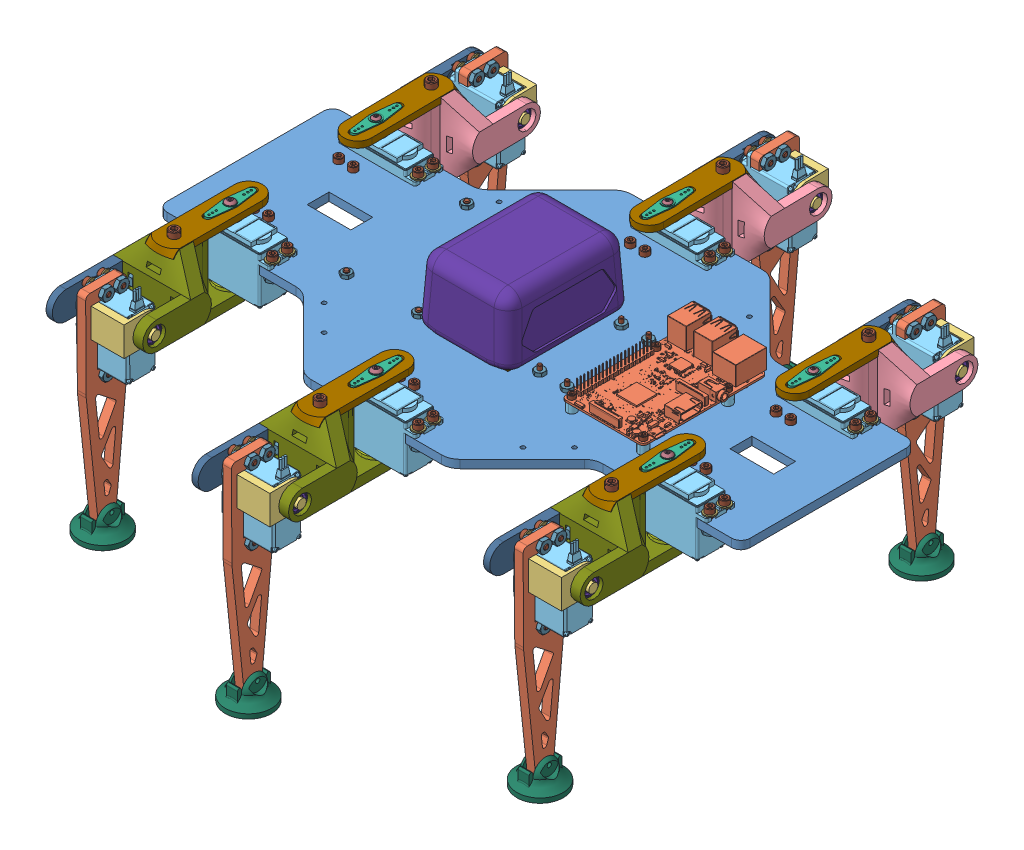
SolidWorks assembly Hexapod, configuration Défaut. Lengths in mm. (continued)
Components (placement in the parent): (continued)
- Battery-1: Battery [Défaut] at (-209.6397 14.6626 -46.247) x (-1 0 0) z (0 0 1) size (64.47 74.3 85.78)
  - MAKITA 4.0AH-1: MAKITA 4.0AH [Défaut] at (0.5853 -29.7874 85.4436) size (64.47 57.15 85.78)
  - MAKITA 4.0AH MOBILE-1: MAKITA 4.0AH MOBILE [Défaut] at (0.5853 -39.3124 91.7936) size (45.84 26.68 66.29)
- arduinoMega-1: arduinoMega [Detailed] at (-270.251 -7.6 40.62) x (0 0 -1) z (-1 0 0) size (108.32 14.5 53.3)
- raspberryPi3B-1: raspberryPi3B [Detailed] at (-112.5 6.35 40) x (0 0 -1) z (0 1 0) size (87.05 58.5 19.5)
- 12Channel PWM-1: 12Channel PWM [Default] at (-160.6 -5.6 40) x (-1 0 0) z (0 0 1) size (25.4 7.55 66.7)
- DROK_090483.stp-1: DROK_090483.stp [Default] at (-90.995 -5.6 69.895) x (-1 0 0) z (0 -1 0) size (50.02 60 18.9)
- socket head cap screw_ai-2: socket head cap screw_ai [HX-SHCS 0.138-32x0.625x0.625-N] at (-54.94 3.5052 69.09) x (0 -1 0) z (1 0 0) size (19.38 5.74 5.74)
- socket head cap screw_ai-3: socket head cap screw_ai [HX-SHCS 0.138-32x0.625x0.625-N] at (-64.94 3.5052 69.09) x (0 -1 0) z (0.5 0 0.866025) size (19.38 5.74 5.74)
- socket head cap screw_ai-4: socket head cap screw_ai [HX-SHCS 0.138-32x0.625x0.625-N] at (-64.94 3.5052 10.91) x (0 -1 0) z (1 0 0) size (19.38 5.74 5.74)
- socket head cap screw_ai-5: socket head cap screw_ai [HX-SHCS 0.138-32x0.625x0.625-N] at (-54.94 3.5052 10.91) x (0 -1 0) z (1 0 0) size (19.38 5.74 5.74)
- socket head cap screw_ai-6: socket head cap screw_ai [HX-SHCS 0.138-32x0.625x0.625-N] at (-214.94 3.5052 119.09) x (0 -1 0) z (1 0 0) size (19.38 5.74 5.74)
- socket head cap screw_ai-7: socket head cap screw_ai [HX-SHCS 0.138-32x0.625x0.625-N] at (-204.94 3.5052 119.09) x (0 -1 0) z (1 0 0) size (19.38 5.74 5.74)
- socket head cap screw_ai-14: socket head cap screw_ai [HX-SHCS 0.138-32x0.625x0.625-N] at (-204.94 3.5052 -39.09) x (0 -1 0) z (1 0 0) size (19.38 5.74 5.74)
- socket head cap screw_ai-15: socket head cap screw_ai [HX-SHCS 0.138-32x0.625x0.625-N] at (-214.94 3.5052 -39.09) x (0 -1 0) z (1 0 0) size (19.38 5.74 5.74)
- socket head cap screw_ai-16: socket head cap screw_ai [HX-SHCS 0.138-32x0.625x0.625-N] at (-354.94 3.5052 69.09) x (0 -1 0) z (1 0 0) size (19.38 5.74 5.74)
- socket head cap screw_ai-17: socket head cap screw_ai [HX-SHCS 0.138-32x0.625x0.625-N] at (-364.94 3.5052 69.09) x (0 -1 0) z (0.5 0 0.866025) size (19.38 5.74 5.74)
- socket head cap screw_ai-18: socket head cap screw_ai [HX-SHCS 0.138-32x0.625x0.625-N] at (-364.94 3.5052 10.91) x (0 -1 0) z (1 0 0) size (19.38 5.74 5.74)
- socket head cap screw_ai-19: socket head cap screw_ai [HX-SHCS 0.138-32x0.625x0.625-N] at (-354.94 3.5052 10.91) x (0 -1 0) z (1 0 0) size (19.38 5.74 5.74)
- machine screw nut hex_ai-60: machine screw nut hex_ai [MSHXNUT 0.138-32-D-N] at (-373.75 -8.4956 -15.08) x (1 0 0) z (0 -1 0) size (7.92 9.15 2.9)
- machine screw nut hex_ai-65: machine screw nut hex_ai [MSHXNUT 0.138-32-D-N] at (-373.75 -8.4956 -4.92) x (1 0 0) z (0 -1 0) size (7.92 9.15 2.9)
- machine screw nut hex_ai-70: machine screw nut hex_ai [MSHXNUT 0.138-32-D-N] at (-326.252 -8.4956 -4.92) x (0.5 0 0.866025) z (0 -1 0) size (7.92 9.15 2.9)
- machine screw nut hex_ai-75: machine screw nut hex_ai [MSHXNUT 0.138-32-D-N] at (-326.252 -8.4956 -15.08) x (0.5 0 0.866025) z (0 -1 0) size (7.92 9.15 2.9)
- machine screw nut hex_ai-80: machine screw nut hex_ai [MSHXNUT 0.138-32-D-N] at (-354.94 -13.5656 10.91) x (0 0 1) z (0 -1 0) size (7.92 9.15 2.9)
- machine screw nut hex_ai-85: machine screw nut hex_ai [MSHXNUT 0.138-32-D-N] at (-364.94 -13.5656 10.91) x (0 0 1) z (0 -1 0) size (7.92 9.15 2.9)
- machine screw nut hex_ai-63: machine screw nut hex_ai [MSHXNUT 0.138-32-D-N] at (-223.75 -8.4956 -65.08) x (1 0 0) z (0 -1 0) size (7.92 9.15 2.9)
- machine screw nut hex_ai-68: machine screw nut hex_ai [MSHXNUT 0.138-32-D-N] at (-223.75 -8.4956 -54.92) x (1 0 0) z (0 -1 0) size (7.92 9.15 2.9)
- machine screw nut hex_ai-73: machine screw nut hex_ai [MSHXNUT 0.138-32-D-N] at (-176.252 -8.4956 -54.92) x (0.5 0 0.866025) z (0 -1 0) size (7.92 9.15 2.9)
- machine screw nut hex_ai-78: machine screw nut hex_ai [MSHXNUT 0.138-32-D-N] at (-176.252 -8.4956 -65.08) x (0.5 0 0.866025) z (0 -1 0) size (7.92 9.15 2.9)
- machine screw nut hex_ai-83: machine screw nut hex_ai [MSHXNUT 0.138-32-D-N] at (-204.94 -13.5656 -39.09) x (0 0 1) z (0 -1 0) size (7.92 9.15 2.9)
- machine screw nut hex_ai-86: machine screw nut hex_ai [MSHXNUT 0.138-32-D-N] at (-214.94 -13.5656 -39.09) x (0 0 1) z (0 -1 0) size (7.92 9.15 2.9)
- machine screw nut hex_ai-87: machine screw nut hex_ai [MSHXNUT 0.138-32-D-N] at (-64.94 -13.5656 10.91) x (0 0 1) z (0 -1 0) size (7.92 9.15 2.9)
- machine screw nut hex_ai-84: machine screw nut hex_ai [MSHXNUT 0.138-32-D-N] at (-54.94 -13.5656 10.91) x (0 0 1) z (0 -1 0) size (7.92 9.15 2.9)
- machine screw nut hex_ai-74: machine screw nut hex_ai [MSHXNUT 0.138-32-D-N] at (-26.252 -8.4956 -4.92) x (0.5 0 0.866025) z (0 -1 0) size (7.92 9.15 2.9)
- machine screw nut hex_ai-79: machine screw nut hex_ai [MSHXNUT 0.138-32-D-N] at (-26.252 -8.4956 -15.08) x (0.5 0 0.866025) z (0 -1 0) size (7.92 9.15 2.9)
- machine screw nut hex_ai-69: machine screw nut hex_ai [MSHXNUT 0.138-32-D-N] at (-73.75 -8.4956 -4.92) x (1 0 0) z (0 -1 0) size (7.92 9.15 2.9)
- machine screw nut hex_ai-64: machine screw nut hex_ai [MSHXNUT 0.138-32-D-N] at (-73.75 -8.4956 -15.08) x (1 0 0) z (0 -1 0) size (7.92 9.15 2.9)
- machine screw nut hex_ai-88: machine screw nut hex_ai [MSHXNUT 0.138-32-D-N] at (-364.94 -10.67 69.09) x (0 0 -1) z (0 1 0) size (7.92 9.15 2.9)
- machine screw nut hex_ai-89: machine screw nut hex_ai [MSHXNUT 0.138-32-D-N] at (-354.94 -10.67 69.09) x (0 0 -1) z (0 1 0) size (7.92 9.15 2.9)
- machine screw nut hex_ai-90: machine screw nut hex_ai [MSHXNUT 0.138-32-D-N] at (-326.252 -5.6 84.92) x (0.5 0 -0.866025) z (0 1 0) size (7.92 9.15 2.9)
- machine screw nut hex_ai-91: machine screw nut hex_ai [MSHXNUT 0.138-32-D-N] at (-326.252 -5.6 95.08) x (0.5 0 -0.866025) z (0 1 0) size (7.92 9.15 2.9)
- machine screw nut hex_ai-92: machine screw nut hex_ai [MSHXNUT 0.138-32-D-N] at (-373.75 -5.6 84.92) x (1 0 0) z (0 1 0) size (7.92 9.15 2.9)
- machine screw nut hex_ai-93: machine screw nut hex_ai [MSHXNUT 0.138-32-D-N] at (-373.75 -5.6 95.08) x (1 0 0) z (0 1 0) size (7.92 9.15 2.9)
- machine screw nut hex_ai-94: machine screw nut hex_ai [MSHXNUT 0.138-32-D-N] at (-223.75 -5.6 145.08) x (1 0 0) z (0 1 0) size (7.92 9.15 2.9)
- machine screw nut hex_ai-95: machine screw nut hex_ai [MSHXNUT 0.138-32-D-N] at (-223.75 -5.6 134.92) x (1 0 0) z (0 1 0) size (7.92 9.15 2.9)
- machine screw nut hex_ai-96: machine screw nut hex_ai [MSHXNUT 0.138-32-D-N] at (-176.252 -5.6 134.92) x (0.5 0 -0.866025) z (0 1 0) size (7.92 9.15 2.9)
- machine screw nut hex_ai-97: machine screw nut hex_ai [MSHXNUT 0.138-32-D-N] at (-176.252 -5.6 145.08) x (0.5 0 -0.866025) z (0 1 0) size (7.92 9.15 2.9)
- machine screw nut hex_ai-98: machine screw nut hex_ai [MSHXNUT 0.138-32-D-N] at (-204.94 -10.67 119.09) x (0 0 -1) z (0 1 0) size (7.92 9.15 2.9)
- machine screw nut hex_ai-99: machine screw nut hex_ai [MSHXNUT 0.138-32-D-N] at (-214.94 -10.67 119.09) x (0 0 -1) z (0 1 0) size (7.92 9.15 2.9)
- machine screw nut hex_ai-100: machine screw nut hex_ai [MSHXNUT 0.138-32-D-N] at (-64.94 -10.67 69.09) x (0 0 -1) z (0 1 0) size (7.92 9.15 2.9)
- machine screw nut hex_ai-101: machine screw nut hex_ai [MSHXNUT 0.138-32-D-N] at (-54.94 -10.67 69.09) x (0 0 -1) z (0 1 0) size (7.92 9.15 2.9)
- machine screw nut hex_ai-102: machine screw nut hex_ai [MSHXNUT 0.138-32-D-N] at (-26.252 -5.6 84.92) x (0.5 0 -0.866025) z (0 1 0) size (7.92 9.15 2.9)
- machine screw nut hex_ai-103: machine screw nut hex_ai [MSHXNUT 0.138-32-D-N] at (-26.252 -5.6 95.08) x (0.5 0 -0.866025) z (0 1 0) size (7.92 9.15 2.9)
- machine screw nut hex_ai-104: machine screw nut hex_ai [MSHXNUT 0.138-32-D-N] at (-73.75 -5.6 84.92) x (1 0 0) z (0 1 0) size (7.92 9.15 2.9)
- machine screw nut hex_ai-105: machine screw nut hex_ai [MSHXNUT 0.138-32-D-N] at (-73.75 -5.6 95.08) x (1 0 0) z (0 1 0) size (7.92 9.15 2.9)
- socket head cap screw_ai-20: socket head cap screw_ai [HX-SHCS 0.138-32x0.5x0.5-N] at (-246.141 -12.6052 74.88) x (0 1 0) z (-0.5 0 -0.866025) size (16.21 5.74 5.74)
- socket head cap screw_ai-21: socket head cap screw_ai [HX-SHCS 0.138-32x0.5x0.5-N] at (-294.361 -12.6052 -6.36) x (0 1 0) z (1 0 0) size (16.21 5.74 5.74)
- socket head cap screw_ai-22: socket head cap screw_ai [HX-SHCS 0.138-32x0.5x0.5-N] at (-246.141 -12.6052 0) x (0 1 0) z (-0.5 0 -0.866025) size (16.21 5.74 5.74)
- socket head cap screw_ai-23: socket head cap screw_ai [HX-SHCS 0.138-32x0.5x0.5-N] at (-294.361 -12.6052 76.11) x (0 1 0) z (-1 0 0) size (16.21 5.74 5.74)
- machine screw nut hex_ai-106: machine screw nut hex_ai [MSHXNUT 0.112-40-D-N] at (-294.361 2.4892 -6.36) x (1 0 0) z (0 1 0) size (6.35 7.33 2.49)
- machine screw nut hex_ai-107: machine screw nut hex_ai [MSHXNUT 0.112-40-D-N] at (-294.361 2.4892 76.11) x (1 0 0) z (0 1 0) size (6.35 7.33 2.49)
- machine screw nut hex_ai-108: machine screw nut hex_ai [MSHXNUT 0.112-40-D-N] at (-246.141 2.4892 0) x (1 0 0) z (0 1 0) size (6.35 7.33 2.49)
- machine screw nut hex_ai-109: machine screw nut hex_ai [MSHXNUT 0.112-40-D-N] at (-246.141 2.4892 74.88) x (1 0 0) z (0 1 0) size (6.35 7.33 2.49)
- socket head cap screw_ai-24: socket head cap screw_ai [HX-SHCS 0.138-32x0.5x0.5-N] at (-130.81 -10.3052 13.48) x (0 1 0) z (-0.5 0 -0.866025) size (16.21 5.74 5.74)
- machine screw nut hex_ai-110: machine screw nut hex_ai [MSHXNUT 0.112-40-D-N] at (-130.81 2.4892 13.48) x (1 0 0) z (0 1 0) size (6.35 7.33 2.49)
- socket head cap screw_ai-25: socket head cap screw_ai [HX-SHCS 0.138-32x0.5x0.5-N] at (-94.18 -10.3052 13.48) x (0 1 0) z (-0.5 0 -0.866025) size (16.21 5.74 5.74)
- socket head cap screw_ai-26: socket head cap screw_ai [HX-SHCS 0.138-32x0.5x0.5-N] at (-130.81 -10.3052 66.31) x (0 1 0) z (-0.5 0 -0.866025) size (16.21 5.74 5.74)
- socket head cap screw_ai-27: socket head cap screw_ai [HX-SHCS 0.138-32x0.5x0.5-N] at (-94.18 -10.3052 66.31) x (0 1 0) z (-0.5 0 -0.866025) size (16.21 5.74 5.74)
- machine screw nut hex_ai-111: machine screw nut hex_ai [MSHXNUT 0.112-40-D-N] at (-94.18 2.4892 13.48) x (1 0 0) z (0 1 0) size (6.35 7.33 2.49)
- machine screw nut hex_ai-112: machine screw nut hex_ai [MSHXNUT 0.112-40-D-N] at (-130.81 2.4892 66.31) x (1 0 0) z (0 1 0) size (6.35 7.33 2.49)
- machine screw nut hex_ai-113: machine screw nut hex_ai [MSHXNUT 0.112-40-D-N] at (-94.18 2.4892 66.31) x (1 0 0) z (0 1 0) size (6.35 7.33 2.49)
- 1_4_Round_Aluminum_Standoff.step-1: 1_4_Round_Aluminum_Standoff.step [Défaut] at (-88 0 21) x (0.963282 0 -0.268492) z (0.268492 0 0.963282) size (6.34 6.36 6.34)
- socket head cap screw_ai-28: socket head cap screw_ai [HX-SHCS 0.112-40x1x0.75-N] at (-88 10.4948 21) x (0 -1 0) z (0.5 0 0.866025) size (28.24 4.65 4.65)
- machine screw nut hex_ai-114: machine screw nut hex_ai [MSHXNUT 0.112-40-D-N] at (-88 -8.0892 21) x (1 0 0) z (0 -1 0) size (6.35 7.33 2.49)
- 1_4_Round_Aluminum_Standoff.step-2: 1_4_Round_Aluminum_Standoff.step [Défaut] at (-137 0 21) x (0.963282 0 -0.268492) z (0.268492 0 0.963282) size (6.34 6.36 6.34)
- 1_4_Round_Aluminum_Standoff.step-3: 1_4_Round_Aluminum_Standoff.step [Défaut] at (-88 0 79) x (0.963282 0 -0.268492) z (0.268492 0 0.963282) size (6.34 6.36 6.34)
- 1_4_Round_Aluminum_Standoff.step-4: 1_4_Round_Aluminum_Standoff.step [Défaut] at (-137 0 79) x (0.963282 0 -0.268492) z (0.268492 0 0.963282) size (6.34 6.36 6.34)
- machine screw nut hex_ai-115: machine screw nut hex_ai [MSHXNUT 0.112-40-D-N] at (-137 -8.0892 21) x (1 0 0) z (0 -1 0) size (6.35 7.33 2.49)
- machine screw nut hex_ai-116: machine screw nut hex_ai [MSHXNUT 0.112-40-D-N] at (-88 -8.0892 79) x (1 0 0) z (0 -1 0) size (6.35 7.33 2.49)
- machine screw nut hex_ai-117: machine screw nut hex_ai [MSHXNUT 0.112-40-D-N] at (-137 -8.0892 79) x (1 0 0) z (0 -1 0) size (6.35 7.33 2.49)
- socket head cap screw_ai-29: socket head cap screw_ai [HX-SHCS 0.112-40x1x0.75-N] at (-137 10.4948 21) x (0 -1 0) z (0.5 0 0.866025) size (28.24 4.65 4.65)
- socket head cap screw_ai-30: socket head cap screw_ai [HX-SHCS 0.112-40x1x0.75-N] at (-88 10.4948 79) x (0 -1 0) z (0.5 0 0.866025) size (28.24 4.65 4.65)
- socket head cap screw_ai-31: socket head cap screw_ai [HX-SHCS 0.112-40x1x0.75-N] at (-137 10.4948 79) x (0 -1 0) z (0.5 0 0.866025) size (28.24 4.65 4.65)
- socket head cap screw_ai-32: socket head cap screw_ai [HX-SHCS 0.112-40x0.5x0.5-N] at (-170 -9.9448 12.05) x (0 1 0) z (-1 0 0) size (15.54 4.65 4.65)
- machine screw nut hex_ai-118: machine screw nut hex_ai [MSHXNUT 0.112-40-D-N] at (-170 2.4892 12.05) x (1 0 0) z (0 1 0) size (6.35 7.33 2.49)
- socket head cap screw_ai-33: socket head cap screw_ai [HX-SHCS 0.112-40x0.5x0.5-N] at (-151.2 -9.9448 12.05) x (0 1 0) z (-1 0 0) size (15.54 4.65 4.65)
- socket head cap screw_ai-34: socket head cap screw_ai [HX-SHCS 0.112-40x0.5x0.5-N] at (-170 -9.9448 67.95) x (0 1 0) z (-1 0 0) size (15.54 4.65 4.65)
- socket head cap screw_ai-35: socket head cap screw_ai [HX-SHCS 0.112-40x0.5x0.5-N] at (-151.2 -9.9448 67.95) x (0 1 0) z (-1 0 0) size (15.54 4.65 4.65)
- machine screw nut hex_ai-119: machine screw nut hex_ai [MSHXNUT 0.112-40-D-N] at (-151.2 2.4892 12.05) x (1 0 0) z (0 1 0) size (6.35 7.33 2.49)
- machine screw nut hex_ai-120: machine screw nut hex_ai [MSHXNUT 0.112-40-D-N] at (-170 2.4892 67.95) x (1 0 0) z (0 1 0) size (6.35 7.33 2.49)
- machine screw nut hex_ai-121: machine screw nut hex_ai [MSHXNUT 0.112-40-D-N] at (-151.2 2.4892 67.95) x (1 0 0) z (0 1 0) size (6.35 7.33 2.49)
Mates (geometry in assembly coordinates):
- Coincident2: coincident anti-aligned: plane of Body-1 through (-370 -5.601 0) normal (0 0 -1)
- Coincident3: coincident aligned: plane of Body-1 through (-400 0 40) normal (0 1 0)
- Coincident4: coincident aligned: plane of Body-1 through (0 0 100) normal (1 0 0)
- Coincident5: coincident anti-aligned: plane of Body-1 through (-400 0 40) normal (0 1 0); plane of Assembly_Leg_V4-1/hs-422-3 through (-50.001 0 -0.094) normal (0 -1 0)
- Concentric3: concentric anti-aligned: cylinder of Body-1 through (-73.75 0 -15.08) axis (0 -1 0) radius 1.45; cylinder of Assembly_Leg_V4-1/hs-422-3 through (-73.75 -26.67 -15.08) axis (0 1 0) radius 2.1844
- Concentric6: concentric aligned: cylinder of Body-1 through (-373.75 -5.601 -4.92) axis (0 1 0) radius 1.45; cylinder of Assembly_Leg_V4-2/hs-422-3 through (-373.75 -26.67 -4.92) axis (0 1 0) radius 2.1844
- Parallel4: parallel anti-aligned: plane of Body-1 through (-370 -5.601 0) normal (0 0 -1); plane of Assembly_Leg_V4-2/hs-422-3 through (-350.001 -5.969 -0.094) normal (0 0 1)
- Coincident9: coincident anti-aligned: plane of Body-1 through (-400 0 40) normal (0 1 0); plane of Assembly_Leg_V4-2/hs-422-3 through (-350.001 0 -0.094) normal (0 -1 0)
- Coincident10: coincident anti-aligned: plane of Body-1 through (-400 0 40) normal (0 1 0); plane of Assembly_Leg_V4-3/hs-422-3 through (-200.001 0 -50.094) normal (0 -1 0)
- Concentric7: concentric anti-aligned: cylinder of Body-1 through (-223.75 0 -54.92) axis (0 -1 0) radius 1.45; cylinder of Assembly_Leg_V4-3/hs-422-3 through (-223.75 -26.67 -54.92) axis (0 1 0) radius 2.1844
- Parallel5: parallel anti-aligned: plane of Body-1 through (-220 -5.6 -50) normal (0 0 -1); plane of Assembly_Leg_V4-3/hs-422-3 through (-200.001 -5.969 -50.094) normal (0 0 1)
- Parallel6: parallel anti-aligned: plane of Body-1 through (-70 -5.6 0) normal (0 0 -1); plane of Assembly_Leg_V4-1/hs-422-3 through (-50.001 -5.969 -0.094) normal (0 0 1)
- Coincident11: coincident anti-aligned: plane of Body-1 through (-400 0 40) normal (0 1 0); plane of Assembly_Leg_V4_Mirror-1/hs-422-3 through (-350.001 0 99.906) normal (0 -1 0)
- Concentric8: concentric aligned: cylinder of Body-1 through (-373.75 -5.601 95.08) axis (0 1 0) radius 1.45; cylinder of Assembly_Leg_V4_Mirror-1/hs-422-3 through (-373.75 -26.67 95.08) axis (0 1 0) radius 2.1844
- Parallel7: parallel anti-aligned: plane of Body-1 through (-370 -5.601 80) normal (0 0 1); plane of Assembly_Leg_V4_Mirror-1/hs-422-3 through (-350.001 -5.969 80.094) normal (0 0 -1)
- Coincident13: coincident anti-aligned: plane of Body-1 through (-400 0 40) normal (0 1 0); plane of Assembly_Leg_V4_Mirror-2/hs-422-3 through (-50.001 0 99.906) normal (0 -1 0)
- Concentric9: concentric anti-aligned: cylinder of Body-1 through (-73.75 0 95.08) axis (0 -1 0) radius 1.45; cylinder of Assembly_Leg_V4_Mirror-2/hs-422-3 through (-73.75 -26.67 95.08) axis (0 1 0) radius 2.1844
- Parallel8: parallel anti-aligned: plane of Body-1 through (-70 -5.6 80) normal (0 0 1); plane of Assembly_Leg_V4_Mirror-2/hs-422-3 through (-50.001 -5.969 80.094) normal (0 0 -1)
- Coincident15: coincident anti-aligned: plane of Body-1 through (-400 0 40) normal (0 1 0); plane of Assembly_Leg_V4_Mirror-3/hs-422-3 through (-200.001 0 149.906) normal (0 -1 0)
- Concentric10: concentric anti-aligned: cylinder of Body-1 through (-223.75 0 145.08) axis (0 -1 0) radius 1.45; cylinder of Assembly_Leg_V4_Mirror-3/hs-422-3 through (-223.75 -26.67 145.08) axis (0 1 0) radius 2.1844
- Parallel9: parallel anti-aligned: plane of Body-1 through (-220 -5.6 130) normal (0 0 1); plane of Assembly_Leg_V4_Mirror-3/hs-422-3 through (-200.001 -5.969 130.094) normal (0 0 -1)
- Coïncidente1: coincident anti-aligned: plane of Body-1 through (-400 0 40) normal (0 1 0); plane of Batterie-1/MAKITA 4.0AH-1 through (-210.225 0 39.1966) normal (0 -1 0)
- Coïncidente2: coincident anti-aligned: plane of arduinoMega-1 through (-270.251 -5.6 40.62) normal (0 1 0); plane of Body-1 through (-400 -5.6 40) normal (0 -1 0)
- Coïncidente4: coincident anti-aligned: plane of Body-1 through (-400 -5.6 40) normal (0 -1 0); plane of 12Channel PWM-1 through (-170 -5.6 12.05) normal (0 1 0)
- Coïncidente5: coincident anti-aligned: plane of Body-1 through (-400 -5.6 40) normal (0 -1 0); plane of DROK_090483.stp-1 through (-112.495 -5.6 39.895) normal (0 1 0)
- Parallèle4: parallel aligned: plane of Body-1 through (0 0 100) normal (1 0 0); plane of 12Channel PWM-1 through (-147.9 -7.1 12.05) normal (1 0 0)
- Concentric13: concentric aligned: cylinder of Body-1 through (-170 0 67.95) axis (0 -1 0) radius 1.25; cylinder of 12Channel PWM-1 through (-170 -2.0645 67.95) axis (0 -1 0) radius 1.25
- Concentric15: concentric aligned: cylinder of Body-1 through (-137 -5.6 21) axis (0 1 0) radius 1.375; cylinder of raspberryPi3B-1 through (-137 6.35 21) axis (0 1 0) radius 1.375
- Concentric16: concentric aligned: cylinder of Body-1 through (-88 -5.6 79) axis (0 1 0) radius 1.375; cylinder of raspberryPi3B-1 through (-88 6.35 79) axis (0 1 0) radius 1.375
- Coincident17: coincident anti-aligned: plane of Body-1 through (-232.45 0 2.16) normal (1 0 0); plane of Batterie-1/MAKITA 4.0AH MOBILE-1 through (-232.45 53.975 45.5466) normal (-1 0 0)
- Coincident18: coincident anti-aligned: plane of Body-1 through (-232.45 0 77.85) normal (0 0 -1); plane of Batterie-1/MAKITA 4.0AH MOBILE-1 through (-192.7625 -22.225 77.85) normal (0 0 1)
- Concentric17: concentric anti-aligned: circle of Body-1; circle of DROK_090483.stp-1
- Concentric18: concentric aligned: cylinder of Body-1 through (-94.18 0 66.31) axis (0 -1 0) radius 1.45; cylinder of DROK_090483.stp-1 through (-94.18 -5.6 66.31) axis (0 -1 0) radius 1.585
- Concentric19: concentric aligned: cylinder of Body-1 through (-246.141 0 0) axis (0 -1 0) radius 1.6; circle of arduinoMega-1
- Concentric22: concentric aligned: cylinder of Body-1 through (-294.361 0 76.11) axis (0 -1 0) radius 1.6; cylinder of arduinoMega-1 through (-294.361 -7.6 76.11) axis (0 -1 0) radius 1.6
- Concentric23: concentric anti-aligned: cylinder of Body-1 through (-54.94 0 69.09) axis (0 -1 0) radius 1.45; cylinder of HX-SHCS 0.138-32x0.625x0.625-N-2 through (-54.94 35.2552 69.09) axis (0 1 0) radius 1.7526
- Concentric24: concentric anti-aligned: cylinder of Body-1 through (-64.94 0 69.09) axis (0 -1 0) radius 1.45; cylinder of HX-SHCS 0.138-32x0.625x0.625-N-3 through (-64.94 35.2552 69.09) axis (0 1 0) radius 1.7526
- Coincident19: coincident anti-aligned: plane of Body-1 through (-400 0 40) normal (0 1 0); plane of HX-SHCS 0.138-32x0.625x0.625-N-2 through (-54.94 0 66.2198) normal (0 -1 0)
- Coincident20: coincident anti-aligned: plane of Body-1 through (-400 0 40) normal (0 1 0); plane of HX-SHCS 0.138-32x0.625x0.625-N-3 through (-62.4543 0 67.6549) normal (0 -1 0)
- Parallel10: parallel aligned: plane of Body-1 through (0 0 100) normal (1 0 0); plane of HX-SHCS 0.138-32x0.625x0.625-N-3 through (-66.3243 1.8796 69.8892) normal (1 0 0)
- Parallel11: parallel aligned: plane of Body-1 through (0 0 100) normal (1 0 0); plane of HX-SHCS 0.138-32x0.625x0.625-N-2 through (-56.3243 1.8796 68.2908) normal (1 0 0)
- Concentric25: concentric anti-aligned: cylinder of Body-1 through (-64.94 0 10.91) axis (0 -1 0) radius 1.45; cylinder of HX-SHCS 0.138-32x0.625x0.625-N-4 through (-64.94 35.2552 10.91) axis (0 1 0) radius 1.7526
- Concentric26: concentric anti-aligned: cylinder of Body-1 through (-54.94 0 10.91) axis (0 -1 0) radius 1.45; cylinder of HX-SHCS 0.138-32x0.625x0.625-N-5 through (-54.94 35.2552 10.91) axis (0 1 0) radius 1.7526
- Coincident23: coincident anti-aligned: plane of Body-1 through (-400 0 40) normal (0 1 0); plane of HX-SHCS 0.138-32x0.625x0.625-N-5 through (-54.94 0 8.0398) normal (0 -1 0)
- Coincident24: coincident anti-aligned: plane of Body-1 through (-400 0 40) normal (0 1 0); plane of HX-SHCS 0.138-32x0.625x0.625-N-4 through (-64.94 0 8.0398) normal (0 -1 0)
- Parallel12: parallel aligned: plane of Body-1 through (0 0 100) normal (1 0 0); plane of HX-SHCS 0.138-32x0.625x0.625-N-5 through (-56.3243 1.8796 10.1108) normal (1 0 0)
- Parallel13: parallel aligned: plane of Body-1 through (0 0 100) normal (1 0 0); plane of HX-SHCS 0.138-32x0.625x0.625-N-4 through (-66.3243 1.8796 10.1108) normal (1 0 0)
- Concentric27: concentric anti-aligned: cylinder of Body-1 through (-214.94 0 -39.09) axis (0 -1 0) radius 1.45; cylinder of HX-SHCS 0.138-32x0.625x0.625-N-13 through (-214.94 40.2807 -39.09) axis (0 1 0) radius 1.7526
- Concentric29: concentric anti-aligned: cylinder of Body-1 through (-204.94 0 119.09) axis (0 -1 0) radius 1.45; cylinder of HX-SHCS 0.138-32x0.625x0.625-N-7 through (-204.94 35.2552 119.09) axis (0 1 0) radius 1.7526
- Concentric30: concentric anti-aligned: cylinder of Body-1 through (-214.94 0 119.09) axis (0 -1 0) radius 1.45; cylinder of HX-SHCS 0.138-32x0.625x0.625-N-6 through (-214.94 35.2552 119.09) axis (0 1 0) radius 1.7526
- Coincident27: coincident anti-aligned: plane of Body-1 through (-400 0 40) normal (0 1 0); plane of HX-SHCS 0.138-32x0.625x0.625-N-7 through (-204.94 0 116.2198) normal (0 -1 0)
- Coincident28: coincident anti-aligned: plane of Body-1 through (-400 0 40) normal (0 1 0); plane of HX-SHCS 0.138-32x0.625x0.625-N-6 through (-214.94 0 116.2198) normal (0 -1 0)
- Parallel14: parallel aligned: plane of Body-1 through (0 0 100) normal (1 0 0); plane of HX-SHCS 0.138-32x0.625x0.625-N-6 through (-216.3243 1.8796 118.2908) normal (1 0 0)
- Parallel15: parallel aligned: plane of Body-1 through (0 0 100) normal (1 0 0); plane of HX-SHCS 0.138-32x0.625x0.625-N-7 through (-206.3243 1.8796 118.2908) normal (1 0 0)
- Concentric31: concentric anti-aligned: cylinder of Body-1 through (-214.94 0 -39.09) axis (0 -1 0) radius 1.45; cylinder of HX-SHCS 0.138-32x0.625x0.625-N-15 through (-214.94 35.2552 -39.09) axis (0 1 0) radius 1.7526
- Concentric32: concentric anti-aligned: cylinder of Body-1 through (-204.94 0 -39.09) axis (0 -1 0) radius 1.45; cylinder of HX-SHCS 0.138-32x0.625x0.625-N-14 through (-204.94 35.2552 -39.09) axis (0 1 0) radius 1.7526
- Coincident31: coincident anti-aligned: plane of Body-1 through (-400 0 40) normal (0 1 0); plane of HX-SHCS 0.138-32x0.625x0.625-N-15 through (-214.94 0 -41.9602) normal (0 -1 0)
- Coincident32: coincident anti-aligned: plane of Body-1 through (-400 0 40) normal (0 1 0); plane of HX-SHCS 0.138-32x0.625x0.625-N-14 through (-204.94 0 -41.9602) normal (0 -1 0)
- Parallel16: parallel anti-aligned: plane of Body-1 through (0 0 100) normal (1 0 0); plane of HX-SHCS 0.138-32x0.625x0.625-N-15 through (-213.5557 1.8796 -38.2908) normal (-1 0 0)
- Parallel17: parallel anti-aligned: plane of Body-1 through (0 0 100) normal (1 0 0); plane of HX-SHCS 0.138-32x0.625x0.625-N-14 through (-203.5557 1.8796 -38.2908) normal (-1 0 0)
- Concentric33: concentric aligned: cylinder of Body-1 through (-364.94 -5.601 69.09) axis (0 1 0) radius 1.45; cylinder of HX-SHCS 0.138-32x0.625x0.625-N-17 through (-364.94 35.2552 69.09) axis (0 1 0) radius 1.7526
- Concentric34: concentric aligned: circle of Body-1; cylinder of HX-SHCS 0.138-32x0.625x0.625-N-16 through (-354.94 35.2552 69.09) axis (0 1 0) radius 1.7526
- Concentric35: concentric aligned: cylinder of Body-1 through (-364.94 -5.601 10.91) axis (0 1 0) radius 1.45; cylinder of HX-SHCS 0.138-32x0.625x0.625-N-18 through (-364.94 35.2552 10.91) axis (0 1 0) radius 1.7526
- Concentric36: concentric aligned: cylinder of Body-1 through (-354.94 -5.601 10.91) axis (0 1 0) radius 1.45; cylinder of HX-SHCS 0.138-32x0.625x0.625-N-19 through (-354.94 35.2552 10.91) axis (0 1 0) radius 1.7526
- Coincident35: coincident anti-aligned: plane of Body-1 through (-400 0 40) normal (0 1 0); plane of HX-SHCS 0.138-32x0.625x0.625-N-18 through (-364.94 0 8.0398) normal (0 -1 0)
- Coincident36: coincident anti-aligned: plane of Body-1 through (-400 0 40) normal (0 1 0); plane of HX-SHCS 0.138-32x0.625x0.625-N-19 through (-354.94 0 8.0398) normal (0 -1 0)
- Coincident37: coincident anti-aligned: plane of Body-1 through (-400 0 40) normal (0 1 0); plane of HX-SHCS 0.138-32x0.625x0.625-N-17 through (-362.4543 0 67.6549) normal (0 -1 0)
- Coincident38: coincident anti-aligned: plane of Body-1 through (-400 0 40) normal (0 1 0); plane of HX-SHCS 0.138-32x0.625x0.625-N-16 through (-354.94 0 66.2198) normal (0 -1 0)
- Parallel18: parallel anti-aligned: plane of Body-1 through (0 0 100) normal (1 0 0); plane of HX-SHCS 0.138-32x0.625x0.625-N-19 through (-353.5557 1.8796 11.7092) normal (-1 0 0)
- Parallel19: parallel anti-aligned: plane of Body-1 through (0 0 100) normal (1 0 0); plane of HX-SHCS 0.138-32x0.625x0.625-N-18 through (-363.5557 1.8796 11.7092) normal (-1 0 0)
- Parallel20: parallel anti-aligned: plane of Body-1 through (0 0 100) normal (1 0 0); plane of HX-SHCS 0.138-32x0.625x0.625-N-16 through (-353.5557 1.8796 69.8892) normal (-1 0 0)
- Parallel21: parallel anti-aligned: plane of Body-1 through (0 0 100) normal (1 0 0); plane of HX-SHCS 0.138-32x0.625x0.625-N-17 through (-363.5557 1.8796 68.2908) normal (-1 0 0)
- Concentric37: concentric anti-aligned: cylinder of Leg-2/socket_1_2_6-32_with_washer-7/HX-SHCS 0.138-32x0.5x0.5-N-1 through (-373.75 38.5826 -15.08) axis (0 1 0) radius 1.7526; circle of MSHXNUT 0.138-32-D-N-1
- Coincident40: coincident anti-aligned: plane of Body-1 through (-400 -5.6 40) normal (0 -1 0); plane of MSHXNUT 0.138-32-D-N-60 through (-373.75 -5.6 -10.5046) normal (0 1 0)
- Parallel22: parallel aligned: plane of Leg-2/hs-422-3 through (-369.94 -5.969 -0.094) normal (-1 0 0); plane of MSHXNUT 0.138-32-D-N-60 through (-377.7124 -5.6 -12.7923) normal (-1 0 0)
- Concentric38: concentric anti-aligned: cylinder of Leg-2/socket_1_2_6-32_with_washer-5/HX-SHCS 0.138-32x0.5x0.5-N-1 through (-373.75 38.5826 -4.92) axis (0 1 0) radius 1.7526; circle of MSHXNUT 0.138-32-D-N-2
- Parallel23: parallel aligned: plane of Leg-2/hs-422-3 through (-369.94 -5.969 -0.094) normal (-1 0 0); plane of MSHXNUT 0.138-32-D-N-65 through (-377.7124 -5.6 -2.6323) normal (-1 0 0)
- Coincident44: coincident anti-aligned: plane of Body-1 through (-400 -5.6 40) normal (0 -1 0); plane of MSHXNUT 0.138-32-D-N-65 through (-373.75 -5.6 -0.3446) normal (0 1 0)
- Coincident45: coincident anti-aligned: cylinder of Leg-2/socket_1_2_6-32_with_washer-8/HX-SHCS 0.138-32x0.5x0.5-N-1 through (-326.252 38.5826 -4.92) axis (0 1 0) radius 1.7526; circle of MSHXNUT 0.138-32-D-N-3
- Concentric40: concentric anti-aligned: cylinder of Leg-2/socket_1_2_6-32_with_washer-6/HX-SHCS 0.138-32x0.5x0.5-N-1 through (-326.252 38.5826 -15.08) axis (0 1 0) radius 1.7526; circle of MSHXNUT 0.138-32-D-N-4
- Coincident47: coincident anti-aligned: plane of Body-1 through (-400 -5.6 40) normal (0 -1 0); plane of MSHXNUT 0.138-32-D-N-55 through (-330.2144 -5.6 -12.7923) normal (0 1 0)
- Coincident48: coincident anti-aligned: plane of Body-1 through (-400 -5.6 40) normal (0 -1 0); plane of MSHXNUT 0.138-32-D-N-3 through (-330.2144 -5.6 -2.6323) normal (0 1 0)
- Parallel24: parallel aligned: plane of Leg-2/hs-422-3 through (-330.062 -5.969 -0.094) normal (1 0 0); plane of MSHXNUT 0.138-32-D-N-55 through (-322.2896 -5.6 -17.3677) normal (1 0 0)
- Parallel25: parallel aligned: plane of Leg-2/hs-422-3 through (-330.062 -5.969 -0.094) normal (1 0 0); plane of MSHXNUT 0.138-32-D-N-3 through (-322.2896 -5.6 -7.2077) normal (1 0 0)
- Concentric41: concentric anti-aligned: cylinder of HX-SHCS 0.138-32x0.625x0.625-N-19 through (-354.94 35.2552 10.91) axis (0 1 0) radius 1.7526; circle of MSHXNUT 0.138-32-D-N-5
- Concentric42: concentric anti-aligned: cylinder of HX-SHCS 0.138-32x0.625x0.625-N-18 through (-364.94 35.2552 10.91) axis (0 1 0) radius 1.7526; circle of MSHXNUT 0.138-32-D-N-6
- Coincident53: coincident anti-aligned: plane of Leg-2/Bearing_mount_leg-1 through (-370.288 -10.67 15) normal (0 -1 0); plane of MSHXNUT 0.138-32-D-N-75 through (-369.5154 -10.67 10.91) normal (0 1 0)
- Coincident54: coincident anti-aligned: plane of Leg-2/Bearing_mount_leg-1 through (-370.288 -10.67 15) normal (0 -1 0); plane of MSHXNUT 0.138-32-D-N-70 through (-359.5154 -10.67 10.91) normal (0 1 0)
- Parallel26: parallel aligned: plane of Leg-2/Bearing_mount_leg-1 through (-370.288 -26.67 5) normal (0 0 1); plane of MSHXNUT 0.138-32-D-N-70 through (-357.2277 -10.67 14.8724) normal (0 0 1)
- Parallel27: parallel aligned: plane of Leg-2/Bearing_mount_leg-1 through (-370.288 -26.67 5) normal (0 0 1); plane of MSHXNUT 0.138-32-D-N-75 through (-367.2277 -10.67 14.8724) normal (0 0 1)
- Concentric43: concentric aligned: cylinder of arduinoMega-1 through (-246.141 -7.6 74.88) axis (0 -1 0) radius 1.6; cylinder of HX-SHCS 0.138-32x0.5x0.5-N-6 through (-246.141 -44.3552 74.88) axis (0 -1 0) radius 1.7526
- Concentric44: concentric aligned: cylinder of arduinoMega-1 through (-294.361 -7.6 76.11) axis (0 -1 0) radius 1.6; cylinder of HX-SHCS 0.138-32x0.5x0.5-N-4 through (-294.361 -44.3552 76.11) axis (0 -1 0) radius 1.7526
- Concentric45: concentric aligned: cylinder of arduinoMega-1 through (-294.361 -7.6 -6.36) axis (0 -1 0) radius 1.6; cylinder of HX-SHCS 0.138-32x0.5x0.5-N-2 through (-294.361 -44.3552 -6.36) axis (0 -1 0) radius 1.7526
- Concentric46: concentric aligned: cylinder of arduinoMega-1 through (-246.141 -7.6 0) axis (0 -1 0) radius 1.6; cylinder of HX-SHCS 0.138-32x0.5x0.5-N-5 through (-246.141 -44.3552 0) axis (0 -1 0) radius 1.7526
- Coincident58: coincident anti-aligned: plane of arduinoMega-1 through (-270.251 -9.1 40.62) normal (0 -1 0); plane of HX-SHCS 0.138-32x0.5x0.5-N-6 through (-243.6553 -9.1 73.4449) normal (0 1 0)
- Coincident59: coincident anti-aligned: plane of arduinoMega-1 through (-270.251 -9.1 40.62) normal (0 -1 0); plane of HX-SHCS 0.138-32x0.5x0.5-N-5 through (-243.6553 -9.1 -1.4351) normal (0 1 0)
- Coincident60: coincident anti-aligned: plane of arduinoMega-1 through (-270.251 -9.1 40.62) normal (0 -1 0); plane of HX-SHCS 0.138-32x0.5x0.5-N-4 through (-294.361 -9.1 73.2398) normal (0 1 0)
- Coincident61: coincident anti-aligned: plane of arduinoMega-1 through (-270.251 -9.1 40.62) normal (0 -1 0); plane of HX-SHCS 0.138-32x0.5x0.5-N-2 through (-294.361 -9.1 -3.4898) normal (0 1 0)
- Concentric47: concentric anti-aligned: cylinder of HX-SHCS 0.138-32x0.5x0.5-N-2 through (-294.361 -44.3552 -6.36) axis (0 -1 0) radius 1.7526; circle of MSHXNUT 0.112-40-S-N-2
- Concentric48: concentric anti-aligned: cylinder of HX-SHCS 0.138-32x0.5x0.5-N-4 through (-294.361 -44.3552 76.11) axis (0 -1 0) radius 1.7526; circle of MSHXNUT 0.112-40-S-N-3
- Concentric49: concentric anti-aligned: cylinder of HX-SHCS 0.138-32x0.5x0.5-N-5 through (-246.141 -44.3552 0) axis (0 -1 0) radius 1.7526; circle of MSHXNUT 0.112-40-S-N-4
- Concentric50: concentric anti-aligned: cylinder of HX-SHCS 0.138-32x0.5x0.5-N-6 through (-246.141 -44.3552 74.88) axis (0 -1 0) radius 1.7526; circle of MSHXNUT 0.112-40-S-N-5
- Coincident62: coincident anti-aligned: plane of Body-1 through (-400 0 40) normal (0 1 0); plane of MSHXNUT 0.112-40-D-N-7 through (-252.491 0 74.88) normal (0 -1 0)
- Coincident63: coincident anti-aligned: plane of Body-1 through (-400 0 40) normal (0 1 0); plane of MSHXNUT 0.112-40-D-N-6 through (-252.491 0 0) normal (0 -1 0)
- Coincident64: coincident anti-aligned: plane of Body-1 through (-400 0 40) normal (0 1 0); plane of MSHXNUT 0.112-40-D-N-5 through (-300.711 0 76.11) normal (0 -1 0)
- Coincident65: coincident anti-aligned: plane of Body-1 through (-400 0 40) normal (0 1 0); plane of MSHXNUT 0.112-40-D-N-4 through (-300.711 0 -6.36) normal (0 -1 0)
- Parallel28: parallel anti-aligned: plane of Body-1 through (-400 0 40) normal (-1 0 0); plane of MSHXNUT 0.112-40-D-N-5 through (-291.186 0 74.2769) normal (1 0 0)
- Parallel30: parallel aligned: plane of Body-1 through (-400 0 40) normal (-1 0 0); plane of MSHXNUT 0.112-40-D-N-4 through (-297.536 0 -8.1931) normal (-1 0 0)
- Parallel31: parallel aligned: plane of Body-1 through (-400 0 40) normal (-1 0 0); plane of MSHXNUT 0.112-40-D-N-6 through (-249.316 0 -1.8331) normal (-1 0 0)
- Parallel32: parallel aligned: plane of Body-1 through (-400 0 40) normal (-1 0 0); plane of MSHXNUT 0.112-40-D-N-7 through (-249.316 0 73.0469) normal (-1 0 0)
- Parallel33: parallel aligned: plane of arduinoMega-1 through (-296.901 -9.1 90.11) normal (-1 0 0); plane of HX-SHCS 0.138-32x0.5x0.5-N-4 through (-292.9767 -10.9796 75.3108) normal (-1 0 0)
- Parallel34: parallel aligned: plane of arduinoMega-1 through (-296.901 -9.1 90.11) normal (-1 0 0); plane of HX-SHCS 0.138-32x0.5x0.5-N-6 through (-244.7567 -10.9796 74.0808) normal (-1 0 0)
- Parallel35: parallel aligned: plane of arduinoMega-1 through (-296.901 -9.1 90.11) normal (-1 0 0); plane of HX-SHCS 0.138-32x0.5x0.5-N-5 through (-244.7567 -10.9796 -0.7992) normal (-1 0 0)
- Parallel36: parallel aligned: plane of arduinoMega-1 through (-296.901 -9.1 90.11) normal (-1 0 0); plane of HX-SHCS 0.138-32x0.5x0.5-N-2 through (-292.9767 -10.9796 -7.1592) normal (-1 0 0)
- Concentric51: concentric aligned: cylinder of DROK_090483.stp-1 through (-130.81 -5.6 13.48) axis (0 -1 0) radius 1.585; cylinder of HX-SHCS 0.138-32x0.5x0.5-N-7 through (-130.81 -42.0552 13.48) axis (0 -1 0) radius 1.7526
- Coincident74: coincident anti-aligned: plane of DROK_090483.stp-1 through (-112.495 -6.8 39.895) normal (0 -1 0); plane of HX-SHCS 0.138-32x0.5x0.5-N-7 through (-128.3243 -6.8 12.0449) normal (0 1 0)
- Parallel37: parallel aligned: plane of DROK_090483.stp-1 through (-133.995 -5.6 69.895) normal (-1 0 0); plane of HX-SHCS 0.138-32x0.5x0.5-N-7 through (-129.4257 -8.6796 12.6808) normal (-1 0 0)
- Concentric52: concentric anti-aligned: cylinder of HX-SHCS 0.138-32x0.5x0.5-N-7 through (-130.81 -42.0552 13.48) axis (0 -1 0) radius 1.7526; circle of MSHXNUT 0.112-40-S-N-6
- Coincident76: coincident anti-aligned: plane of Body-1 through (-400 0 40) normal (0 1 0); plane of MSHXNUT 0.112-40-D-N-8 through (-137.16 0 13.48) normal (0 -1 0)
- Parallel38: parallel anti-aligned: plane of Body-1 through (0 0 100) normal (1 0 0); plane of MSHXNUT 0.112-40-D-N-8 through (-133.985 0 11.6469) normal (-1 0 0)
- Concentric53: concentric anti-aligned: cylinder of Body-1 through (-88 -5.6 21) axis (0 1 0) radius 1.375; cylinder of 1_4_Round_Aluminum_Standoff.step-1 through (-88 6.35 21) axis (0 -1 0) radius 3.1712
- Coincident78: coincident anti-aligned: plane of Body-1 through (-400 0 40) normal (0 1 0); plane of 1_4_Round_Aluminum_Standoff.step-1 through (-88 0 21) normal (0 -1 0)
- Coincident79: coincident anti-aligned: plane of raspberryPi3B-1 through (-112.5 6.35 40) normal (0 -1 0); plane of 1_4_Round_Aluminum_Standoff.step-1 through (-88 6.35 21) normal (0 1 0)
- Concentric54: concentric aligned: cylinder of raspberryPi3B-1 through (-88 6.35 21) axis (0 1 0) radius 1.375; cylinder of HX-SHCS 0.112-40x1x0.75-N-8 through (-88 42.2448 21) axis (0 1 0) radius 1.4224
- Coincident80: coincident anti-aligned: plane of raspberryPi3B-1 through (-112.5 7.65 40) normal (0 1 0); plane of HX-SHCS 0.112-40x1x0.75-N-8 through (-85.9873 7.65 19.8379) normal (0 -1 0)
- Parallel39: parallel aligned: plane of raspberryPi3B-1 through (-84.5 7.65 82.5) normal (1 0 0); plane of HX-SHCS 0.112-40x1x0.75-N-8 through (-89.1938 9.1994 21.6892) normal (1 0 0)
- Concentric55: concentric anti-aligned: cylinder of HX-SHCS 0.112-40x1x0.75-N-8 through (-88 42.2448 21) axis (0 1 0) radius 1.4224; circle of MSHXNUT 0.112-40-D-N-3
- Coincident83: coincident anti-aligned: plane of Body-1 through (-400 -5.6 40) normal (0 -1 0); plane of MSHXNUT 0.112-40-D-N-3 through (-94.35 -5.6 21) normal (0 1 0)
- Parallel40: parallel aligned: plane of Body-1 through (0 0 100) normal (1 0 0); plane of MSHXNUT 0.112-40-D-N-3 through (-84.825 -5.6 22.8331) normal (1 0 0)
- Concentric56: concentric aligned: cylinder of 12Channel PWM-1 through (-170 -2.0645 12.05) axis (0 -1 0) radius 1.25; cylinder of HX-SHCS 0.112-40x0.5x0.5-N-9 through (-170 -41.6948 12.05) axis (0 -1 0) radius 1.4224
- Coincident85: coincident anti-aligned: plane of 12Channel PWM-1 through (-170 -7.1 12.05) normal (0 -1 0); plane of HX-SHCS 0.112-40x0.5x0.5-N-9 through (-170 -7.1 9.7259) normal (0 1 0)
- Parallel41: parallel aligned: plane of 12Channel PWM-1 through (-147.9 -7.1 12.05) normal (1 0 0); plane of HX-SHCS 0.112-40x0.5x0.5-N-9 through (-171.1938 -8.6494 12.7392) normal (1 0 0)
- Concentric57: concentric anti-aligned: cylinder of HX-SHCS 0.112-40x0.5x0.5-N-9 through (-170 -41.6948 12.05) axis (0 -1 0) radius 1.4224; circle of MSHXNUT 0.112-40-D-N-68
- Coincident88: coincident anti-aligned: plane of Body-1 through (-400 0 40) normal (0 1 0); plane of MSHXNUT 0.112-40-D-N-68 through (-176.35 0 12.05) normal (0 -1 0)
- Parallel42: parallel aligned: plane of Body-1 through (0 0 100) normal (1 0 0); plane of MSHXNUT 0.112-40-D-N-68 through (-166.825 0 10.2169) normal (1 0 0)
